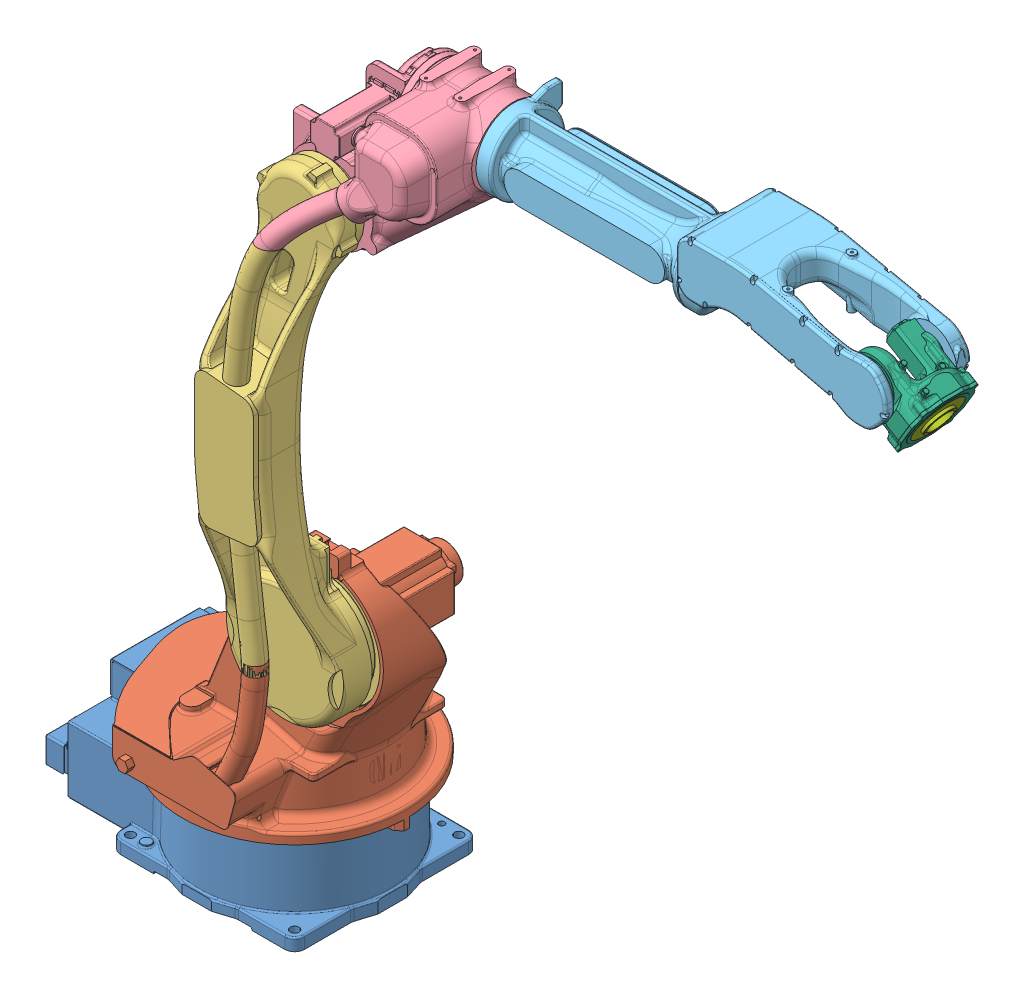
SolidWorks assembly MA2010-PROTO-2, configuration 默认. Lengths in mm.
Overall size (1744.29 1565 496.61).
7 component instances, 7 part files, 6 mates.
Components (placement in the parent):
- BASE_AXIS-1: BASE_AXIS [默认] at origin size (595.7 208.2 395.46)
- S_AXIS-1: S_AXIS [默认] at origin size (522.02 516 496.61)
- L_AXIS-1: L_AXIS [默认] at origin size (259.19 969.49 187.73)
- U_AXIS-1: U_AXIS [默认] at origin size (422.63 424.1 381.03)
- R_AXIS-1: R_AXIS [默认] at origin size (847.16 178.3 179.99)
- B_AXIS-1: B_AXIS [默认] at (-576.8251 838.7406 0) x (0.858597 -0.512651 0) z (0 0 1) size (148.8 137.51 133.24)
- T_AXIS-1: T_AXIS [默认] at (-576.8251 838.7406 0) x (0.858597 -0.512651 0) z (0 0 1) size (12.6 100 100)
Mates (geometry in assembly coordinates):
- 同心1: concentric aligned: cylinder of B_AXIS-1 through (1312.7081 1416.8108 0) axis (0.858597 -0.512651 0) radius 50; cylinder of T_AXIS-1 through (1302.9845 1422.6166 0) axis (0.858597 -0.512651 0) radius 50
- 重合1: coincident aligned: plane of B_AXIS-1 through (1312.7081 1416.8108 0) normal (0.858597 -0.512651 0); plane of T_AXIS-1 through (1312.7081 1416.8108 0) normal (0.858597 -0.512651 0)
- 同心2: concentric anti-aligned: cylinder of R_AXIS-1 through (1232 1465 59.6) axis (0 0 1) radius 38; cylinder of B_AXIS-1 through (1232 1465 64.45) axis (0 0 -1) radius 35
- 重合3: coincident anti-aligned: plane of R_AXIS-1 through (1232 1465 -64) normal (0 0 1); plane of B_AXIS-1 through (1351.9582 1475.7203 -64) normal (0 0 -1)
- 距离1: distance = 2 mm anti-aligned: plane of U_AXIS-1 through (445 1560 -100) normal (1 0 0); plane of R_AXIS-1 through (447 1465 0) normal (-1 0 0)
- 同心3: concentric aligned: cylinder of U_AXIS-1 through (457.9 1465 0) axis (-1 0 0) radius 77; cylinder of R_AXIS-1 through (857 1465 0) axis (-1 0 0) radius 77
